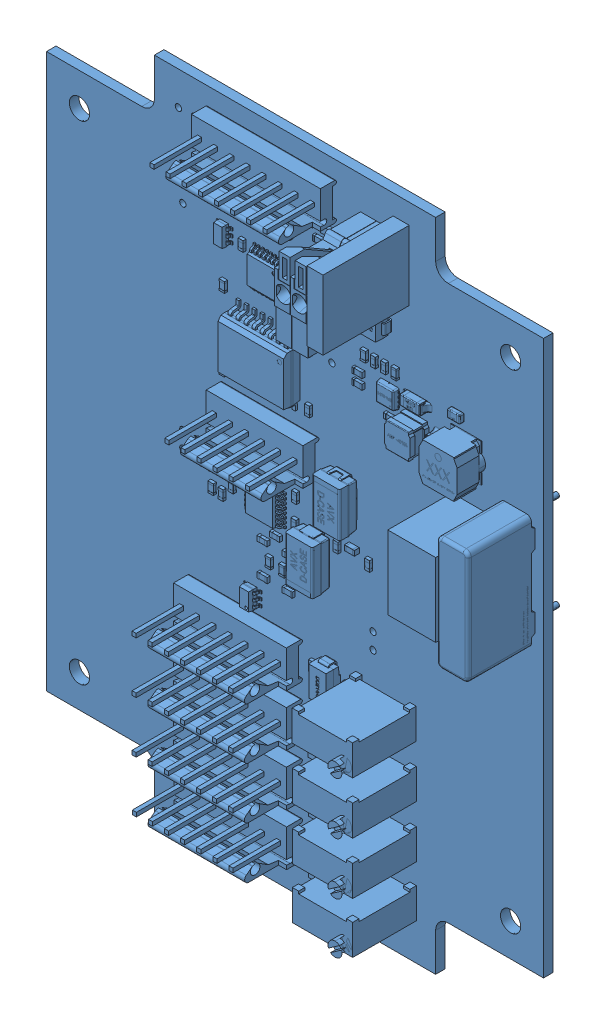
SolidWorks assembly PCB_VelvetADCv.2, configuration Default. Lengths in mm.
Overall size (78.38 103.38 22.57).
10 component instances, 4 part files, 9 mates.
Components (placement in the parent):
- g212mf-g311mf^PCB_VelvetADCv.2-1: g212mf-g311mf^PCB_VelvetADCv.2 [Default] at origin size (91.63 145 55.04) (hidden, virtual)
  - G212-COVER^g212mf-g311mf_PCB_VelvetADCv.2-1: G212-COVER^g212mf-g311mf_PCB_VelvetADCv.2 [Default] at (92211.1548 46503.1602 -30.4904) size (90 115 15) (virtual)
  - G212-BASE^g212mf-g311mf_PCB_VelvetADCv.2-1: G212-BASE^g212mf-g311mf_PCB_VelvetADCv.2 [Default] at (92211.1548 46503.1602 -30.4904) size (91.63 145 41.54) (virtual)
- Velvet ADC v2.0^PCB_VelvetADCv.2-1: Velvet ADC v2.0^PCB_VelvetADCv.2 [Default] at (-36.9584 48.4354 -12.2277) x (0 -1 0) z (0 0 1) size (103.38 78.38 22.57) (virtual)
- GX16-4P-1: GX16-4P [Default] at (-76.7536 24.3509 2.2242) x (0.999848 0 -0.017452) z (0.015171 -0.494331 0.869141) size (47.5 21.45 18.91) (hidden)
- GX16-4P-2: GX16-4P [Default] at (-76.6976 -24.4662 5.4308) x (0.999848 0 -0.017452) z (0.015084 -0.503008 0.86415) size (47.5 21.45 18.91) (hidden)
- GX16-4P-3: GX16-4P [Default] at (81.2229 24.8878 1.8754) x (-0.999848 0 -0.017452) z (0.014253 -0.577133 -0.816526) size (47.5 21.45 18.91) (hidden)
- GX16-4P-4: GX16-4P [Default] at (-76.7629 -0.092 1.6932) x (0.999848 0 -0.017452) z (0.016683 0.293639 0.955771) size (47.5 21.45 18.91) (hidden)
- GX16-4P-5: GX16-4P [Default] at (2.5366 -94.6692 6.5565) x (0 0.999848 -0.017452) z (-0.995263 0.001697 0.097201) size (47.5 21.45 18.91) (hidden)
- GX16-4P-6: GX16-4P [Default] at (81.1944 -21.6203 3.5074) x (-0.999848 0 -0.017452) z (0.017281 0.139867 -0.99002) size (47.5 21.45 18.91) (hidden)
Mates (geometry in assembly coordinates):
- Coincident1: coincident anti-aligned: plane of g212mf-g311mf^СБ_VelvetADCv.2-1/G212-BASE^g212mf-g311mf_СБ_VelvetADCv.2-1 through (-31.7684 35.2404 -13.7277) normal (0 0 1); plane of Velvet ADC v2.0.step-1 through (2.2316 -3.2546 -13.7277) normal (0 0 -1)
- Concentric1: concentric aligned: circle of g212mf-g311mf.step-1/G212-BASE.step-1; circle of Velvet ADC v2.0.step-1
- Parallel1: parallel aligned: line of g212mf-g311mf^СБ_VelvetADCv.2-1/G212-BASE^g212mf-g311mf_СБ_VelvetADCv.2-1 through (43.9088 -45.2596 -17.7277) axis (0 1 0); line of Velvet ADC v2.0.step-1 through (41.4216 -46.9296 -12.2277) axis (0 1 0)
- Coincident2: coincident anti-aligned: plane of g212mf-g311mf^СБ_VelvetADCv.2-1/G212-BASE^g212mf-g311mf_СБ_VelvetADCv.2-1 through (-43.4491 -54.6938 -20.7297) normal (-0.999848 0 0.017452); plane of GX16-4P-1 through (-42.9811 32.1743 6.0844) normal (0.999848 0 -0.017452)
- Coincident3: coincident anti-aligned: plane of g212mf-g311mf^СБ_VelvetADCv.2-1/G212-BASE^g212mf-g311mf_СБ_VelvetADCv.2-1 through (-43.4491 -54.6938 -20.7297) normal (-0.999848 0 0.017452); plane of GX16-4P-4 through (-43.1141 8.5113 -1.5373) normal (0.999848 0 -0.017452)
- Coincident4: coincident anti-aligned: plane of g212mf-g311mf^СБ_VelvetADCv.2-1/G212-BASE^g212mf-g311mf_СБ_VelvetADCv.2-1 through (-43.4491 -54.6938 -20.7297) normal (-0.999848 0 0.017452); plane of GX16-4P-2 through (-42.9237 -16.6876 9.369) normal (0.999848 0 -0.017452)
- Coincident5: coincident anti-aligned: plane of g212mf-g311mf^СБ_VelvetADCv.2-1/G212-BASE^g212mf-g311mf_СБ_VelvetADCv.2-1 through (47.9124 48.1746 -20.7297) normal (0.999848 0 0.017452); plane of GX16-4P-3 through (47.6187 32.2377 -3.9062) normal (-0.999848 0 -0.017452)
- Coincident6: coincident anti-aligned: plane of g212mf-g311mf^СБ_VelvetADCv.2-1/G212-BASE^g212mf-g311mf_СБ_VelvetADCv.2-1 through (47.9124 48.1746 -20.7297) normal (0.999848 0 0.017452); plane of GX16-4P-6 through (47.4776 -12.7088 4.1778) normal (-0.999848 0 -0.017452)
- Coincident8: coincident anti-aligned: plane of g212mf-g311mf^СБ_VelvetADCv.2-1/G212-BASE^g212mf-g311mf_СБ_VelvetADCv.2-1 through (2.2316 -60.7596 18.2703) normal (0 -0.999848 0.017452); plane of GX16-4P-5 through (1.6617 -61.1307 -2.9877) normal (0 0.999848 -0.017452)
